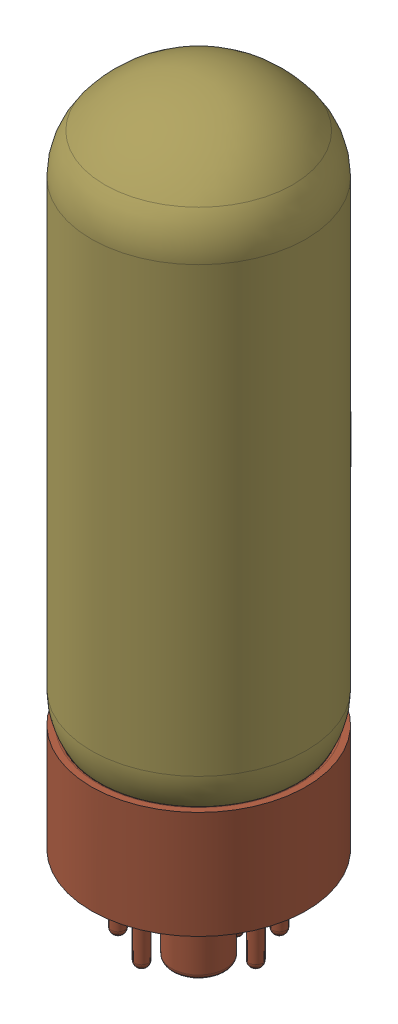
SolidWorks assembly el34 assembly_r1, configuration Default. Lengths in mm.
Overall size (47.19 113.85 47.19).
20 component instances, 13 part files, 49 mates.
Components (placement in the parent):
- el34 mica_r1-1: el34 mica_r1 [Default] at origin size (26.4 1.54 30.07)
- el34 cathode_r1-1: el34 cathode_r1 [Default] x (0 0 1) z (-1 0 0) size (9.5 47.57 7.12)
- el34 g2_r1-1: el34 g2_r1 [Default] x (0 0 1) z (-1 0 0) size (11.34 51.5 5.09)
- el34 suppressor_r1-1: el34 suppressor_r1 [Default] x (0 0 -1) z (1 0 0) size (16.21 51 11.14)
- el34 anode rod_r1-1: el34 anode rod_r1 [Default] at (-9.8 0 0) size (1 50 1)
- el34 anode rod_r1-2: el34 anode rod_r1 [Default] at (9.8 0 0) size (1 50 1)
- el34 anode_r1-1: el34 anode_r1 [Default] at (0 20.5 0) size (27 41 9.26)
- el34 mica_r1-2: el34 mica_r1 [Default] at (0 41.3 0) size (26.4 1.54 30.07)
- el34 g1 support_r1-1: el34 g1 support_r1 [Default] x (0 0 1) z (-1 0 0) size (7.11 56.7 3.01)
- el34 anode_r1-2: el34 anode_r1 [Default] at (0 20.5 0) x (-1 0 0) z (0 0 -1) size (27 41 9.26)
- el34 anode fixing_r1-1: el34 anode fixing_r1 [Default] at (9.8 41.3 0) x (0 0 1) z (-1 0 0) size (6 3 0.66)
- el34 anode fixing_r1-2: el34 anode fixing_r1 [Default] at (-9.8 41.3 0) x (0 0 -1) z (1 0 0) size (6 3 0.66)
- el34 anode fixing_r1-3: el34 anode fixing_r1 [Default] at (-9.8 -3.3 0) x (0 0 -1) z (1 0 0) size (6 3 0.66)
- el34 anode fixing_r1-4: el34 anode fixing_r1 [Default] at (9.8 -3.3 0) x (0 0 1) z (-1 0 0) size (6 3 0.66)
- el34 grid brace_r1-1: el34 grid brace_r1 [Default] at (0 41.3 0) x (0 0 -1) z (1 0 0) size (7.41 8 12.48)
- el34 boat_r1-1: el34 boat_r1 [Default] at (0 53.8 -1.4) x (-1 0 0) z (0 0 -1) size (13.25 13.4 13.83)
- el34 octal_base_r1-1: el34 octal_base_r1 [Default] at (0 -25.65 0) x (-1 0 0) z (0 0 -1) size (32 30.2 32)
- el34 envelope_r1-1: el34 envelope_r1 [Default] at (0 -14 0) x (-0.707107 0 -0.707107) z (0.707107 0 -0.707107) size (32.07 105.5 34.67)
  - el34 glass_r1-1: el34 glass_r1 [Default] at origin size (38.82 100 34.67)
  - el34 pins out of envelope_r1-1: el34 pins out of envelope_r1 [Default] x (0.92388 0 -0.382683) z (0.382683 0 0.92388) size (16.97 31 16.97)
Mates (geometry in assembly coordinates):
- Coincident1: coincident aligned: plane of el34 mica_r1-1 through (0 0 0) normal (0 1 0); plane of el34 cathode_r1-1 through (0 0 0) normal (0 1 0)
- Coincident2: coincident aligned: plane of el34 mica_r1-1 through (0 0 0) normal (0 0 1); plane of el34 cathode_r1-1 through (0 0 0) normal (0 0 1)
- Coincident3: coincident anti-aligned: plane of el34 mica_r1-1 through (0 0 0) normal (1 0 0); plane of el34 cathode_r1-1 through (0 0 0) normal (-1 0 0)
- Coincident4: coincident aligned: plane of el34 g2_r1-1 through (0 0 0) normal (0 0 1); plane of el34 mica_r1-1 through (0 0 0) normal (0 0 1)
- Coincident5: coincident aligned: plane of el34 mica_r1-1 through (0 0 0) normal (0 1 0); plane of el34 g2_r1-1 through (0 0 0) normal (0 1 0)
- Coincident6: coincident anti-aligned: plane of el34 g2_r1-1 through (0 0 0) normal (-1 0 0); plane of assembly through (0 0 0) normal (1 0 0)
- Coincident7: coincident aligned: plane of el34 mica_r1-1 through (0 0 0) normal (0 1 0); plane of el34 suppressor_r1-1 through (0 0 0) normal (0 1 0)
- Coincident8: coincident anti-aligned: plane of el34 suppressor_r1-1 through (0 0 0) normal (0 0 -1); plane of assembly through (0 0 0) normal (0 0 1)
- Coincident9: coincident aligned: plane of el34 suppressor_r1-1 through (0 0 0) normal (1 0 0); plane of assembly through (0 0 0) normal (1 0 0)
- Coincident10: coincident aligned: plane of el34 mica_r1-1 through (0 0 0) normal (0 1 0); plane of el34 anode rod_r1-1 through (-9.8 0 0) normal (0 1 0)
- Concentric1: concentric aligned: cylinder of el34 mica_r1-1 through (-9.8 -9.8 0) axis (0 1 0) radius 0.5; cylinder of el34 anode rod_r1-1 through (-9.8 -4.5 0) axis (0 1 0) radius 0.5
- Coincident11: coincident aligned: plane of el34 mica_r1-1 through (0 0 0) normal (0 1 0); plane of el34 anode rod_r1-2 through (9.8 0 0) normal (0 1 0)
- Concentric2: concentric aligned: cylinder of el34 mica_r1-1 through (9.8 -9.8 0) axis (0 1 0) radius 0.5; cylinder of el34 anode rod_r1-2 through (9.8 -4.5 0) axis (0 1 0) radius 0.5
- Coincident12: coincident aligned: plane of el34 suppressor_r1-1 through (0 0 0) normal (1 0 0); plane of el34 anode_r1-1 through (0 20.5 0) normal (1 0 0)
- Coincident13: coincident aligned: plane of el34 anode_r1-1 through (0 20.5 0) normal (0 0 1); plane of assembly through (0 0 0) normal (0 0 1)
- Coincident16: coincident anti-aligned: plane of el34 anode_r1-1 through (-10.666 0 -0.5) normal (0 -1 0); plane of assembly through (0 0 0) normal (0 1 0)
- Coincident17: coincident anti-aligned: plane of el34 anode_r1-1 through (-10.666 41 -0.5) normal (0 1 0); plane of el34 mica_r1-2 through (0 41 0) normal (0 -1 0)
- Coincident18: coincident aligned: plane of el34 mica_r1-2 through (0 41.3 0) normal (0 0 1); plane of assembly through (0 0 0) normal (0 0 1)
- Coincident19: coincident aligned: plane of el34 mica_r1-2 through (0 41.3 0) normal (1 0 0); plane of assembly through (0 0 0) normal (1 0 0)
- Coincident20: coincident aligned: plane of el34 mica_r1-1 through (0 0 0) normal (0 1 0); plane of el34 g1 support_r1-1 through (0 0 0) normal (0 1 0)
- Coincident21: coincident anti-aligned: plane of el34 g1 support_r1-1 through (0 0 0) normal (-1 0 0); plane of assembly through (0 0 0) normal (1 0 0)
- Coincident22: coincident aligned: plane of el34 g1 support_r1-1 through (0 0 0) normal (0 0 1); plane of assembly through (0 0 0) normal (0 0 1)
- Coincident23: coincident anti-aligned: plane of el34 anode_r1-2 through (0 20.5 0) normal (0 0 -1); plane of assembly through (0 0 0) normal (0 0 1)
- Coincident24: coincident anti-aligned: plane of el34 anode_r1-2 through (0 20.5 0) normal (-1 0 0); plane of assembly through (0 0 0) normal (1 0 0)
- Coincident25: coincident anti-aligned: plane of el34 mica_r1-1 through (0 0 0) normal (0 1 0); plane of el34 anode_r1-2 through (10.666 0 0.5) normal (0 -1 0)
- Concentric3: concentric anti-aligned: cylinder of el34 anode rod_r1-2 through (9.8 -4.5 0) axis (0 1 0) radius 0.5; cylinder of el34 anode fixing_r1-1 through (9.8 44.3 0) axis (0 -1 0) radius 0.5
- Concentric4: concentric anti-aligned: cylinder of el34 anode rod_r1-1 through (-9.8 -4.5 0) axis (0 1 0) radius 0.5; cylinder of el34 anode fixing_r1-2 through (-9.8 44.3 0) axis (0 -1 0) radius 0.5
- Coincident26: coincident anti-aligned: plane of el34 mica_r1-2 through (0 41.3 0) normal (0 1 0); plane of el34 anode fixing_r1-2 through (-10 41.3 -0.6708) normal (0 -1 0)
- Coincident27: coincident anti-aligned: plane of el34 mica_r1-2 through (0 41.3 0) normal (0 1 0); plane of el34 anode fixing_r1-1 through (10 41.3 0.6708) normal (0 -1 0)
- Parallel1: parallel aligned: plane of el34 anode fixing_r1-2 through (-9.8 44.3 -0.6708) normal (1 0 0); plane of assembly through (0 0 0) normal (1 0 0)
- Parallel2: parallel anti-aligned: plane of el34 anode fixing_r1-1 through (9.8 44.3 0.6708) normal (-1 0 0); plane of assembly through (0 0 0) normal (1 0 0)
- Coincident30: coincident anti-aligned: plane of el34 mica_r1-1 through (0 -0.3 0) normal (0 -1 0); plane of el34 anode fixing_r1-3 through (-10 -0.3 -0.6708) normal (0 1 0)
- Coincident31: coincident anti-aligned: plane of el34 mica_r1-1 through (0 -0.3 0) normal (0 -1 0); plane of el34 anode fixing_r1-4 through (10 -0.3 0.6708) normal (0 1 0)
- Concentric5: concentric anti-aligned: cylinder of el34 anode rod_r1-1 through (-9.8 -4.5 0) axis (0 1 0) radius 0.5; cylinder of el34 anode fixing_r1-3 through (-9.8 -0.3 0) axis (0 -1 0) radius 0.5
- Concentric6: concentric anti-aligned: cylinder of el34 anode rod_r1-2 through (9.8 -4.5 0) axis (0 1 0) radius 0.5; cylinder of el34 anode fixing_r1-4 through (9.8 -0.3 0) axis (0 -1 0) radius 0.5
- Parallel3: parallel anti-aligned: plane of el34 anode fixing_r1-4 through (9.8 -0.3 0.6708) normal (-1 0 0); plane of assembly through (0 0 0) normal (1 0 0)
- Parallel4: parallel aligned: plane of el34 anode fixing_r1-3 through (-9.8 -0.3 3) normal (1 0 0); plane of assembly through (0 0 0) normal (1 0 0)
- Coincident34: coincident aligned: plane of el34 mica_r1-2 through (0 41.3 0) normal (0 1 0); plane of el34 grid brace_r1-1 through (0 41.3 0) normal (0 1 0)
- Coincident35: coincident anti-aligned: plane of el34 grid brace_r1-1 through (0 41.3 0) normal (0 0 -1); plane of assembly through (0 0 0) normal (0 0 1)
- Coincident36: coincident aligned: plane of el34 grid brace_r1-1 through (0 41.3 0) normal (1 0 0); plane of assembly through (0 0 0) normal (1 0 0)
- Coincident37: coincident anti-aligned: plane of el34 mica_r1-2 through (0 41.3 0) normal (0 1 0); plane of el34 boat_r1-1 through (0 41.3 -8.3) normal (0 -1 0)
- Coincident38: coincident anti-aligned: plane of el34 boat_r1-1 through (0 53.8 -1.4) normal (-1 0 0); plane of assembly through (0 0 0) normal (1 0 0)
- Distance1: distance = 1.4 mm anti-aligned: plane of el34 boat_r1-1 through (0 53.8 -1.4) normal (0 0 -1); plane of assembly through (0 0 0) normal (0 0 1)
- Coincident43: coincident aligned: line of el34 envelope_r1-1/el34 glass_r1-1 through (123.5606 0 -48.9442) axis (0 0 1)
- Coincident45: coincident aligned: line of el34 octal_base_r1-1 through (39.6 0 -41.45) axis (0 0 1); line of el34 envelope_r1-1/el34 glass_r1-1 through (123.5606 0 -48.9442) axis (0 0 1)
- Coincident49: coincident aligned: plane of el34 octal_base_r1-1 through (0 -25.65 0) normal (-0.92388 0 -0.382683); plane of el34 envelope_r1-1/el34 pins out of envelope_r1-1 through (0 -14 0) normal (-0.92388 0 -0.382683)
- Distance2: distance = 11.65 mm aligned: plane of el34 envelope_r1-1/el34 pins out of envelope_r1-1 through (0 -14 0) normal (0 1 0); plane of el34 octal_base_r1-1 through (0 -25.65 0) normal (0 1 0)
- Coincident51: coincident anti-aligned: plane of el34 octal_base_r1-1 through (0 -25.65 0) normal (-1 0 0); plane of assembly through (0 0 0) normal (1 0 0)
- Distance3: distance = 14 mm aligned: plane of el34 envelope_r1-1 through (0 -14 0) normal (0 1 0); plane of assembly through (0 0 0) normal (0 1 0)
